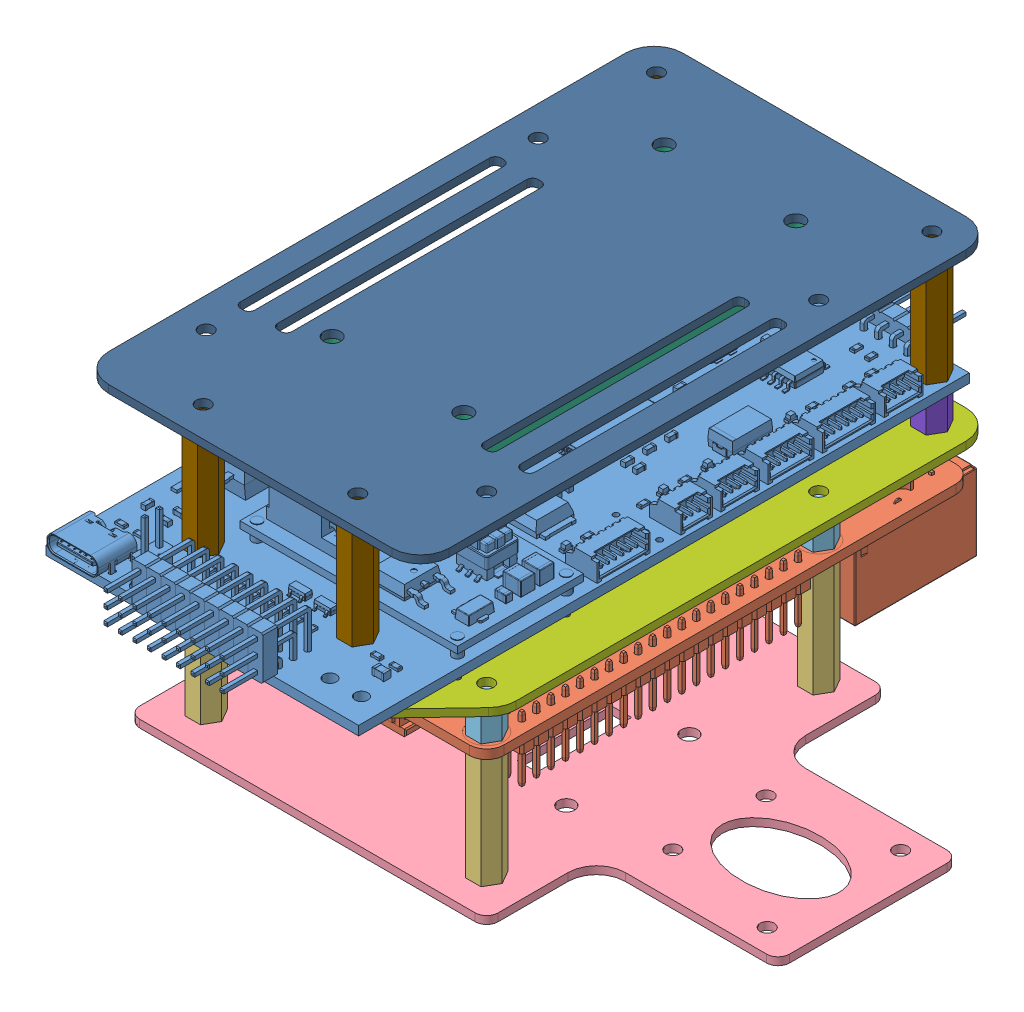
SolidWorks assembly Electronics_stack, configuration Default. Lengths in mm.
Overall size (126 63.9 122.32).
22 component instances, 10 part files, 36 mates.
Components (placement in the parent):
- OSAVC_simplified-1: OSAVC_simplified [Default] at (-27.305 36.55 53.34) x (0 0 -1) z (0 1 0) size (122.32 54.61 12.15)
- Raspberry_Pi_4B-2: Raspberry_Pi_4B [Default] at (0 20.8 -10.84) x (0 0 -1) z (-1 0 0) size (89 19.92 58.4)
- M2.5_hex_stand_20mm-1: M2.5_hex_stand_20mm [Default] at (24.5 0 28.16) size (5.43 26 4.7)
- M2.5_hex_stand_20mm-2: M2.5_hex_stand_20mm [Default] at (24.5 0 -29.84) size (5.43 26 4.7)
- M2.5_hex_stand_20mm-3: M2.5_hex_stand_20mm [Default] at (-24.5 0 28.16) size (5.43 26 4.7)
- M2.5_hex_stand_20mm-4: M2.5_hex_stand_20mm [Default] at (-24.5 0 -29.84) size (5.43 26 4.7)
- Top_plate_electronics-1: Top_plate_electronics [Default] at origin size (126 1.35 69.93)
- M2.5_hex_stand_6mm-1: M2.5_hex_stand_6mm [Default] at (24.5 21.6 28.16) size (5.43 11.72 4.7)
- M2.5_hex_stand_6mm-2: M2.5_hex_stand_6mm [Default] at (24.5 21.6 -29.84) size (5.43 11.72 4.7)
- M2.5_hex_stand_6mm-3: M2.5_hex_stand_6mm [Default] at (-24.5 21.6 28.16) size (5.43 11.72 4.7)
- M2.5_hex_stand_6mm-4: M2.5_hex_stand_6mm [Default] at (-24.5 21.6 -29.84) size (5.43 11.72 4.7)
- Coral_USB_accelerator-1: Coral_USB_accelerator [Default] at (-16 48.55 21.66) x (0 0 -1) z (1 0 0) size (65 8 30)
- Stack_plate_osavc_pi-1: Stack_plate_osavc_pi [Default] at (0 27.6 0) x (1 0 0) z (0 0 -1) size (59.5 1.35 100.3)
- M2.5_hex_stand_6mm_f-f-1: M2.5_hex_stand_6mm_f-f [Default] at (13.515 28.95 39.7) size (5.43 6 4.7)
- M2.5_hex_stand_6mm_f-f-2: M2.5_hex_stand_6mm_f-f [Default] at (-13.485 28.95 39.7) size (5.43 6 4.7)
- M2.5_hex_stand_6mm_f-f-3: M2.5_hex_stand_6mm_f-f [Default] at (24.015 28.95 -50.1) size (5.43 6 4.7)
- M2.5_hex_stand_6mm_f-f-4: M2.5_hex_stand_6mm_f-f [Default] at (-24.085 28.95 -50.1) size (5.43 6 4.7)
- M2.5_hex_stand_20mm_f-f-1: M2.5_hex_stand_20mm_f-f [Default] at (13.515 36.55 39.7) size (5.43 20 4.7)
- M2.5_hex_stand_20mm_f-f-2: M2.5_hex_stand_20mm_f-f [Default] at (-13.485 36.55 39.7) size (5.43 20 4.7)
- M2.5_hex_stand_20mm_f-f-3: M2.5_hex_stand_20mm_f-f [Default] at (24.015 36.55 -50.1) size (5.43 20 4.7)
- M2.5_hex_stand_20mm_f-f-4: M2.5_hex_stand_20mm_f-f [Default] at (-24.085 36.55 -50.1) size (5.43 20 4.7)
- Stack_plate_osavc_coral-1: Stack_plate_osavc_coral [Default] at (0 56.55 0) size (59.5 1.35 100.3)
Mates (geometry in assembly coordinates):
- Parallel3: parallel anti-aligned: plane of OSAVC_simplified-1 through (0 34.95 0) normal (0 -1 0)
- Coincident12: coincident aligned: plane of OSAVC_simplified-1 through (0 36.55 53.34) normal (1 0 0)
- Coincident13: coincident anti-aligned: plane of OSAVC_simplified-1 through (-27.305 36.55 0) normal (0 0 -1)
- Coincident17: coincident anti-aligned: plane of Raspberry_Pi_4B-2 through (0 20.8 -10.84) normal (-1 0 0)
- Parallel5: parallel anti-aligned: plane of Raspberry_Pi_4B-2 through (0 20 -10.84) normal (0 -1 0)
- Coincident19: coincident: line of Raspberry_Pi_4B-2 through (-25 21.6 -53.34) axis (1 0 0)
- Concentric1: concentric anti-aligned: cylinder of Raspberry_Pi_4B-2 through (24.5 20 28.16) axis (0 -1 0) radius 1.35; cylinder of M2.5_hex_stand_20mm-1 through (24.5 -6 28.16) axis (0 1 0) radius 1.25
- Coincident20: coincident anti-aligned: plane of M2.5_hex_stand_20mm-1 through (24.5 0 28.16) normal (0 -1 0)
- Coincident21: coincident anti-aligned: plane of Raspberry_Pi_4B-2 through (0 20 -10.84) normal (0 -1 0); plane of M2.5_hex_stand_20mm-1 through (24.5 20 28.16) normal (0 1 0)
- Parallel6: parallel aligned: plane of M2.5_hex_stand_20mm-1 through (24.5 0 28.16) normal (1 0 0)
- Coincident23: coincident aligned: plane of Top_plate_electronics-1 through (0 0 0) normal (0 1 0)
- Coincident24: coincident aligned: plane of Top_plate_electronics-1 through (0 0 0) normal (1 0 0)
- Coincident25: coincident aligned: plane of Top_plate_electronics-1 through (0 0 0) normal (0 0 1)
- Concentric2: concentric anti-aligned: cylinder of Raspberry_Pi_4B-2 through (24.5 20 28.16) axis (0 -1 0) radius 1.35; cylinder of M2.5_hex_stand_6mm-1 through (24.5 15.6 28.16) axis (0 1 0) radius 1.25
- Coincident26: coincident anti-aligned: plane of Raspberry_Pi_4B-2 through (0 21.6 -10.84) normal (0 1 0); plane of M2.5_hex_stand_6mm-1 through (24.5 21.6 28.16) normal (0 -1 0)
- Parallel7: parallel aligned: plane of M2.5_hex_stand_6mm-1 through (24.5 21.6 28.16) normal (1 0 0)
- Coincident27: coincident aligned: plane of Raspberry_Pi_4B-2 through (-1 20.8 -10.84) normal (1 0 0); plane of Coral_USB_accelerator-1 through (-1 48.55 21.66) normal (1 0 0)
- Parallel8: parallel anti-aligned: plane of Coral_USB_accelerator-1 through (-1 48.55 -10.84) normal (0 -1 0)
- Coincident33: coincident anti-aligned: plane of M2.5_hex_stand_6mm-4 through (-24.5 27.6 -29.84) normal (0 1 0); plane of Stack_plate_osavc_pi-1 through (0 27.6 0) normal (0 -1 0)
- Coincident34: coincident anti-aligned: plane of Stack_plate_osavc_pi-1 through (0 27.6 0) normal (0 0 -1)
- Coincident35: coincident aligned: plane of Stack_plate_osavc_pi-1 through (0 27.6 0) normal (1 0 0)
- Concentric4: concentric anti-aligned: cylinder of Stack_plate_osavc_pi-1 through (13.515 28.95 39.7) axis (0 -1 0) radius 1.25; cylinder of M2.5_hex_stand_6mm_f-f-1 through (13.515 34.95 39.7) axis (0 1 0) radius 1.025
- Coincident38: coincident anti-aligned: plane of Stack_plate_osavc_pi-1 through (0 28.95 0) normal (0 1 0); plane of M2.5_hex_stand_6mm_f-f-1 through (13.515 28.95 39.7) normal (0 -1 0)
- Parallel9: parallel aligned: plane of M2.5_hex_stand_6mm_f-f-1 through (13.515 28.95 39.7) normal (1 0 0)
- Concentric5: concentric anti-aligned: cylinder of Stack_plate_osavc_pi-1 through (24.015 28.95 -50.1) axis (0 -1 0) radius 1.25; cylinder of M2.5_hex_stand_6mm_f-f-3 through (24.015 34.95 -50.1) axis (0 1 0) radius 1.025
- Coincident40: coincident anti-aligned: plane of Stack_plate_osavc_pi-1 through (0 28.95 0) normal (0 1 0); plane of M2.5_hex_stand_6mm_f-f-3 through (24.015 28.95 -50.1) normal (0 -1 0)
- Parallel10: parallel aligned: plane of M2.5_hex_stand_6mm_f-f-3 through (24.015 28.95 -50.1) normal (1 0 0)
- Coincident42: coincident anti-aligned: plane of OSAVC_simplified-1 through (0 34.95 0) normal (0 -1 0); plane of M2.5_hex_stand_6mm_f-f-1 through (13.515 34.95 39.7) normal (0 1 0)
- Coincident43: coincident anti-aligned: plane of OSAVC_simplified-1 through (0 36.55 0) normal (0 1 0); plane of M2.5_hex_stand_20mm_f-f-1 through (13.515 36.55 39.7) normal (0 -1 0)
- Concentric6: concentric aligned: cylinder of OSAVC_simplified-1 through (13.515 36.55 39.7) axis (0 1 0) radius 1.35; cylinder of M2.5_hex_stand_20mm_f-f-1 through (13.515 56.55 39.7) axis (0 1 0) radius 1.025
- Parallel11: parallel aligned: plane of M2.5_hex_stand_20mm_f-f-1 through (13.515 36.55 39.7) normal (1 0 0)
- Coincident45: coincident aligned: plane of Coral_USB_accelerator-1 through (-1 56.55 -10.84) normal (0 1 0); plane of M2.5_hex_stand_20mm_f-f-2 through (-13.485 56.55 39.7) normal (0 1 0)
- Distance1: distance = 10 mm anti-aligned: plane of Coral_USB_accelerator-1 through (-1 52.55 -43.34) normal (0 0 -1)
- Coincident47: coincident aligned: plane of M2.5_hex_stand_20mm_f-f-4 through (-24.085 56.55 -50.1) normal (0 1 0); plane of Part1^Electronics_stack-1 through (0 56.55 0) normal (0 1 0)
- Coincident48: coincident aligned: plane of Part1^Electronics_stack-1 through (0 56.55 0) normal (0 0 1)
- Coincident49: coincident aligned: plane of Part1^Electronics_stack-1 through (0 56.55 0) normal (1 0 0)
